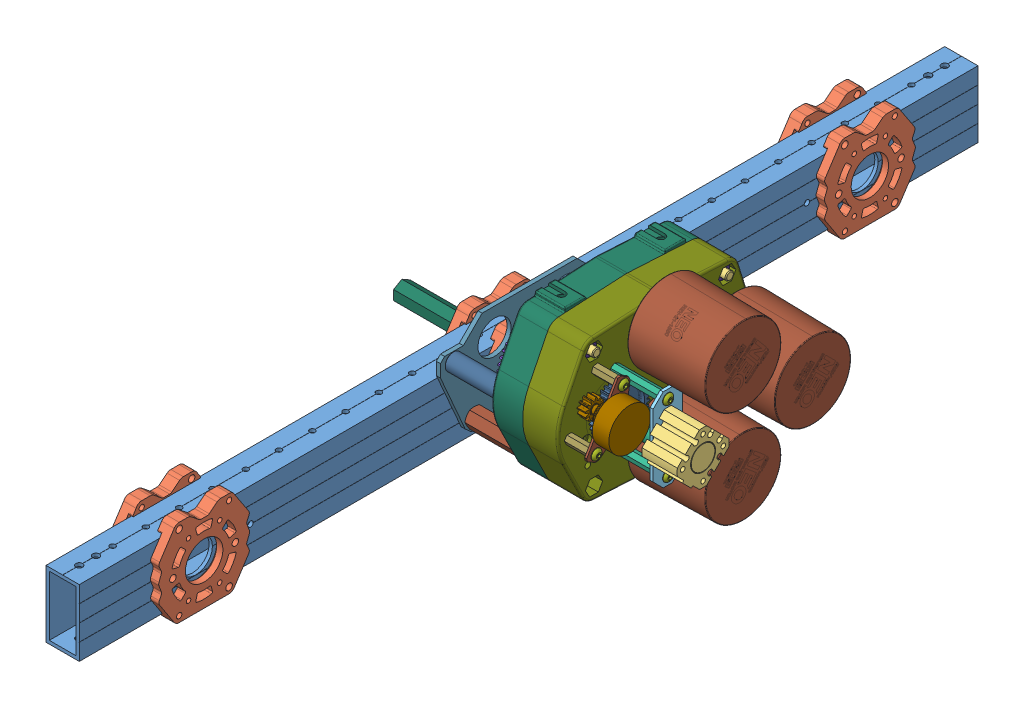
SolidWorks assembly Copy of 2020IR.subassembly_drivebase_gearbox_wheels_mounted.originaldownload.osears, configuration Default. Lengths in mm.
Overall size (265.36 166.93 685.8).
117 component instances, 65 part files, 0 mates.
Components (placement in the parent):
- 217-8000-001-002_mod_to_1_x_2_x_0_100_Pre-Drilled_VersaFrame_Aluminum_Tube_(27)_217-3453.drp-1: 217-8000-001-002_mod_to_1_x_2_x_0_100_Pre-Drilled_VersaFrame_Aluminum_Tube_(27)_217-3453.drp [Default] at (-12.7 22.86 749.3) size (25.4 50.8 685.8)
- VersaBlock_Kit_217-3432.drp-1: VersaBlock_Kit_217-3432.drp [Default] at (1.5875 24.5237 596.8746) x (0 0 -1) z (1 0 0) size (69.4 66.32 9.53)
- VersaBlock_Kit_217-3432.drp-2: VersaBlock_Kit_217-3432.drp [Default] at (1.5875 24.5237 342.8746) x (0 0 -1) z (1 0 0) size (69.4 66.32 9.53)
- VersaBlock_Kit_217-3432.drp-3: VersaBlock_Kit_217-3432.drp [Default] at (1.5875 24.5237 88.8746) x (0 0 -1) z (1 0 0) size (69.4 66.32 9.53)
- VersaBlock_Kit_217-3432.drp-4: VersaBlock_Kit_217-3432.drp [Default] at (-26.9875 24.5237 88.8746) x (0 0 1) z (-1 0 0) size (69.4 66.32 9.53)
- VersaBlock_Kit_217-3432.drp-5: VersaBlock_Kit_217-3432.drp [Default] at (-26.9875 24.5237 342.8746) x (0 0 1) z (-1 0 0) size (69.4 66.32 9.53)
- VersaBlock_Kit_217-3432.drp-6: VersaBlock_Kit_217-3432.drp [Default] at (-26.9875 24.5237 596.8746) x (0 0 1) z (-1 0 0) size (69.4 66.32 9.53)
- 3_CIM_Ball_Shifter_Base_Kit_with_WCD_3rd_Stage_217-3269_With_NEO.drp-1: 3_CIM_Ball_Shifter_Base_Kit_with_WCD_3rd_Stage_217-3269_With_NEO.drp [Default] at (101.2952 62.8142 378.4138) x (0 1 0) z (-1 0 0) size (166.93 180.09 265.36)
  - 3_CIM_Ball_Shifter_Base_Kit_with_WCD_3rd_Stage_217-3269.STEP-1: 3_CIM_Ball_Shifter_Base_Kit_with_WCD_3rd_Stage_217-3269.STEP [Default] at origin size (154.62 161.2 265.36)
    - 217-2778-001 Rev2_NCQ8A075-050M.STEP-1: 217-2778-001 Rev2_NCQ8A075-050M.STEP [Default] at (0 0 -53.848) x (-0.707107 0.707107 0) z (0 0 1) size (31.75 33.34 39.88)
      - 217-2778-NCQ8A075-050M_NCQ8 Tube_075A.STEP-1: 217-2778-NCQ8A075-050M_NCQ8 Tube_075A.STEP [Default] at origin size (31.75 33.34 26.92)
      - 217-2778-NCQ8A075-050M_NCQ8 Rod_075M.STEP-1: 217-2778-NCQ8A075-050M_NCQ8 Rod_075M.STEP [Default] at (0 0 -8.85) x (0.866025 -0.5 0) z (0 0 1) size (18.95 18.95 35.27)
      - 217-2778-NCQ8A075-050M_Snap Ring_075.STEP-1: 217-2778-NCQ8A075-050M_Snap Ring_075.STEP [Default] at (0 0 10.362) size (21 20.74 0.97)
    - 217-4098-100 Rev1.STEP-1: 217-4098-100 Rev1.STEP [Default] at (0 0 -16.927) x (-0.503316 0.864103 0) z (0 0 1) size (18.03 19.79 22.46)
      - 217-4098-006 Rev2.STEP-1: 217-4098-006 Rev2.STEP [Default] at (0 0 -4.6312) x (0 -1 0) z (0 0 -1) size (18.09 11.02 22.46)
      - 217-4098-006 Rev2.STEP-2: 217-4098-006 Rev2.STEP [Default] at (0 0 -4.6312) x (0 1 0) z (0 0 -1) size (18.09 11.02 22.46)
      - 217-3489-001 Rev1.STEP-1: 217-3489-001 Rev1.STEP [Default] at (0 0 -4.6312) x (0 0 1) z (-0.980217 -0.197926 0) size (4.77 12.7 12.7)
      - 97633A130_97633A130_grv.STEP-1: 97633A130_97633A130_grv.STEP [Default] at (0 0 -7.33) x (0 0 -1) z (0.979861 0.199683 0) size (0.64 8.74 7.34)
      - 91251A107_91251A107.STEP-1: 91251A107_91251A107.STEP [Default] at (-4.8375 -6.735 -9.4343) x (0 0.863883 -0.503692) z (-1 0 0) size (4.65 4.65 10.79)
      - 91251A107_91251A107.STEP-2: 91251A107_91251A107.STEP [Default] at (4.8375 6.735 -9.4343) x (0 0.470889 -0.882193) z (1 0 0) size (4.65 4.65 10.79)
    - 217-3288-001 Rev3.STEP-1: 217-3288-001 Rev3.STEP [Default] at (0 0 0.0889) x (0.055929 -0.998435 0) z (0 0 1) size (99.51 99.53 98.3)
      - 217-4099-000 Rev2_high gear.STEP-1: 217-4099-000 Rev2_high gear.STEP [Default] x (-1 0 0) z (0 0 1) size (22.23 22.23 98.3)
        - 217-4098-005 Rev1_91612A226.STEP-1: 217-4098-005 Rev1_91612A226.STEP [Default] at (0 0 46.2661) x (-0.144757 0 0.989467) z (0 -1 0) size (3.02 3.15 18.22)
        - 217-4098-003 Rev2.STEP-1: 217-4098-003 Rev2.STEP [Default] x (1 0 0) z (0 0 -1) size (22.23 22.23 55.94)
        - 217-4099-002 Rev3.STEP-1: 217-4099-002 Rev3.STEP [Default] at (0 0 53.467) x (0 0 1) z (-1 0 0) size (40.96 12.73 14.67)
        - 217-4098-004 Rev1.STEP-1: 217-4098-004 Rev1.STEP [Default] at (0 0 14.2494) x (0.873474 -0.48687 0) z (0 0 1) size (11.68 11.68 56)
      - 217-3212-101 Rev1.STEP-1: 217-3212-101 Rev1.STEP [Default] at (-11.5751 10.4131 45.3224) x (0.923728 0.383049 0) z (0 0 -1) size (46.46 46.56 12.7)
        - 217-2428-022 Rev1.STEP-1: 217-2428-022 Rev1.STEP [Default] at (6.7035 14.0527 24.6087) size (28.57 28.57 6.1)
        - 217-3212-001 Rev1_34t.STEP-1: 217-3212-001 Rev1_34t.STEP [Default] at (6.7035 14.0527 27.9107) size (46.46 46.56 11.11)
      - 217-3222-101 Rev1.STEP-1: 217-3222-101 Rev1.STEP [Default] at (21.0941 -5.2804 52.7371) x (-0.889163 -0.457591 0) z (0 0 -1) size (73.87 73.92 12.7)
        - 217-2428-022 Rev1.STEP-1: 217-2428-022 Rev1.STEP [Default] at (16.3398 14.3476 19.3234) size (28.57 28.57 6.1)
        - 217-3222-001 Rev1_Spur01.STEP-1: 217-3222-001 Rev1_Spur01.STEP [Default] at (16.3398 14.3476 22.6254) x (0.999377 0.0353 0) z (0 0 1) size (71.39 71.45 11.11)
      - 217-2428-008 Rev2.STEP-1: 217-2428-008 Rev2.STEP [Default] at (0 0 10.2679) size (31.75 31.75 1.59)
      - 217-2428-028 Rev1_97633A250.STEP-1: 217-2428-028 Rev1_97633A250.STEP [Default] at (0 0 37.1221) x (0 0 1) z (0.9357 -0.352797 0) size (1.07 23.39 21.18)
      - 217-2428-007 Rev1.STEP-1: 217-2428-007 Rev1.STEP [Default] at (7.809 4.5085 14.2494) x (-0.69071 0.455693 -0.561483) z (-0.67559 -0.683536 0.276329) size (6.35 6.35 6.35)
      - 217-2428-007 Rev1.STEP-2: 217-2428-007 Rev1.STEP [Default] at (5.4343 3.1375 26.9494) x (-0.162331 -0.978398 0.128005) z (0.857281 -0.204076 -0.472676) size (6.35 6.35 6.35)
      - 217-2428-007 Rev1.STEP-3: 217-2428-007 Rev1.STEP [Default] at (-5.4343 3.1375 26.9494) x (0.928483 0.348617 0.128005) z (-0.251905 0.844465 -0.472676) size (6.35 6.35 6.35)
      - 217-2428-007 Rev1.STEP-4: 217-2428-007 Rev1.STEP [Default] at (0 -6.275 26.9494) x (-0.766153 0.629782 0.128005) z (-0.605376 -0.640389 -0.472676) size (6.35 6.35 6.35)
      - 217-2428-007 Rev1.STEP-5: 217-2428-007 Rev1.STEP [Default] at (-7.809 4.5085 14.2494) x (-0.049287 -0.826019 -0.561483) z (0.929754 -0.24331 0.276329) size (6.35 6.35 6.35)
      - 217-2428-007 Rev1.STEP-6: 217-2428-007 Rev1.STEP [Default] at (0 -9.017 14.2494) x (0.739997 0.370326 -0.561483) z (-0.254164 0.926846 0.276329) size (6.35 6.35 6.35)
    - 217-2733-001 Rev2.STEP-1: 217-2733-001 Rev2.STEP [Default] at (0 53.4162 37.6682) x (0 0 1) z (-0.00054 -1 0) size (7.11 24.61 24.61)
    - 217-2733-001 Rev2.STEP-2: 217-2733-001 Rev2.STEP [Default] at (0 53.4162 7.9248) x (0 0 -1) z (-0.038475 0.99926 0) size (7.11 24.61 24.61)
    - 217-2731-001 Rev2.STEP-1: 217-2731-001 Rev2.STEP [Default] at (0 0 0.0381) x (-0.099212 0.995066 0) z (0.995066 0.099212 0) size (31.12 7.94 31.12)
    - 217-2789-001 Rev2.STEP-1: 217-2789-001 Rev2.STEP [Default] at (0 0 43.2943) x (0 0 -1) z (-0.58471 0.811243 0) size (11.1 38.4 38.4)
    - 217-2428-012 Rev2.STEP-1: 217-2428-012 Rev2.STEP [Default] at (0 0 -40.386) size (63.5 22.23 2.29)
    - 217-2428-005 Rev1.STEP-1: 217-2428-005 Rev1.STEP [Default] at (25.4 0 -19.05) x (-0.557362 -0.83027 0) z (-0.83027 0.557362 0) size (7.33 38.98 6.35)
    - 217-2428-005 Rev1.STEP-2: 217-2428-005 Rev1.STEP [Default] at (-25.4 0 -19.05) x (0.667436 0.744667 0) z (0.744667 -0.667436 0) size (7.33 38.98 6.35)
    - SCREW-832-0375.STEP-1: SCREW-832-0375.STEP [Default] at (25.4 0 -42.5958) x (0 0 1) z (-0.875404 0.483392 0) size (11.73 7.92 7.92)
    - SCREW-832-0375.STEP-2: SCREW-832-0375.STEP [Default] at (-25.4 0 -42.5958) x (0 0 1) z (-0.966319 0.257347 0) size (11.73 7.92 7.92)
    - SCREW-832-0375.STEP-3: SCREW-832-0375.STEP [Default] at (25.4 0 5.3848) x (0 0 -1) z (1 0 0) size (11.73 7.92 7.92)
    - SCREW-832-0375.STEP-4: SCREW-832-0375.STEP [Default] at (-25.4 0 5.3848) x (0 0 -1) z (0.941463 -0.337115 0) size (11.73 7.92 7.92)
    - SBS1_SBS-0632-0250.STEP-1: SBS1_SBS-0632-0250.STEP [Default] at (15.494 0 -36.2458) x (0 0 -1) z (0.854303 -0.519775 0) size (8.57 6.68 6.65)
    - SBS1_SBS-0632-0250.STEP-2: SBS1_SBS-0632-0250.STEP [Default] at (-15.494 0 -36.2458) x (0 0 -1) z (0.854303 -0.519775 0) size (8.57 6.68 6.65)
    - 217-2428-017 Rev2.STEP-1: 217-2428-017 Rev2.STEP [Default] at (12.7 -21.997 -3.614) x (-0.578458 -0.815712 0) z (0 0 -1) size (14.73 14.73 7.37)
    - 217-2428-016 Rev3_Spur01.STEP-1: 217-2428-016 Rev3_Spur01.STEP [Default] at (0 0 -3.614) x (0.873157 -0.48744 0) z (0 0 1) size (40.67 40.74 13.32)
    - 217-2428-019 Rev1.STEP-1: 217-2428-019 Rev1.STEP [Default] at (12.7 -21.997 -20.6248) x (0.866025 0.5 0) z (0 0 1) size (50.8 19.05 1.57)
    - 217-2428-006 Rev1.STEP-1: 217-2428-006 Rev1.STEP [Default] at (32.079 -14.2875 -9.525) x (-0.752416 0.658689 0) z (0.658689 0.752416 0) size (7.33 19.93 6.35)
    - 217-2428-006 Rev1.STEP-2: 217-2428-006 Rev1.STEP [Default] at (-3.6662 -34.925 -9.525) x (0.84498 0.534798 0) z (0.534798 -0.84498 0) size (7.33 19.93 6.35)
    - SCREW-832-0375.STEP-5: SCREW-832-0375.STEP [Default] at (32.079 -14.2875 4.7498) x (0 0 -1) z (0.980613 0.195955 0) size (11.73 7.92 7.92)
    - SCREW-832-0375.STEP-6: SCREW-832-0375.STEP [Default] at (-3.6662 -34.925 5.3848) x (0 0 -1) z (-0.672515 -0.740083 0) size (11.73 7.92 7.92)
    - SCREW-832-0375.STEP-7: SCREW-832-0375.STEP [Default] at (-3.6662 -34.925 -22.8346) x (0 0 1) z (0.948865 0.315681 0) size (11.73 7.92 7.92)
    - SCREW-832-0375.STEP-8: SCREW-832-0375.STEP [Default] at (32.079 -14.2875 -22.8346) x (0 0 1) z (-0.875404 0.483392 0) size (11.73 7.92 7.92)
    - 217-2614-001_12t.STEP-1: 217-2614-001_12t.STEP [Default] at (36.9798 39.6868 15.8623) x (-0.087156 0.996195 0) z (0 0 1) size (18.29 18.29 19)
    - 217-2761-001 rev1.STEP-1: 217-2761-001 rev1.STEP [Default] at (33.1943 39.3556 16.1) x (0.087156 -0.996195 0) z (0 0 1) size (2 2 20)
    - 217-2761-001 rev1.STEP-2: 217-2761-001 rev1.STEP [Default] at (-40.7653 40.018 16.1) x (0.087156 0.996195 0) z (0 0 1) size (2 2 20)
    - 217-2614-001_12t.STEP-2: 217-2614-001_12t.STEP [Default] at (-36.9798 39.6868 15.8623) x (0.087156 0.996195 0) z (0 0 1) size (18.29 18.29 19)
    - 217-2614-001_12t.STEP-3: 217-2614-001_12t.STEP [Default] at (0 92.8624 15.8623) x (0.97459 0.223996 0) z (0 0 1) size (18.29 18.29 19)
    - 217-2761-001 rev1.STEP-3: 217-2761-001 rev1.STEP [Default] at (-0.8512 96.5658 16.1) x (0.97459 0.223996 0) z (0 0 1) size (2 2 20)
    - 217-3195-002 rev2.STEP-1: 217-3195-002 rev2.STEP [Default] at (0 0 50.546) x (-1 0 0) z (0 0 -1) size (114.31 152.24 24.96)
    - 217-3195-001 Rev1.STEP-1: 217-3195-001 Rev1.STEP [Default] at origin size (113.41 152.24 26.86)
    - Nylock Nut_NNY2520-ZC.STEP-1: Nylock Nut_NNY2520-ZC.STEP [Default] at (48.8823 73.025 37.846) x (0 0.866025 -0.5) z (-1 0 0) size (12.85 11.89 7.62)
    - Nylock Nut_NNY2520-ZC.STEP-2: Nylock Nut_NNY2520-ZC.STEP [Default] at (48.8823 -3.175 37.846) x (0 0 -1) z (-1 0 0) size (12.85 11.89 7.62)
    - Nylock Nut_NNY2520-ZC.STEP-3: Nylock Nut_NNY2520-ZC.STEP [Default] at (44.45 85.725 7.8613) x (0 1 0) z (0 0 -1) size (12.85 11.89 7.62)
    - 276-1027-001.STEP-1: 276-1027-001.STEP [Default] at (47.625 58.1787 6.35) x (0 1 0) z (-1 0 0) size (8.61 5.64 9.94)
    - 276-1027-001.STEP-2: 276-1027-001.STEP [Default] at (-47.625 58.1787 6.35) x (0 -1 0) z (1 0 0) size (8.61 5.64 9.94)
    - SCREW-832-1750.STEP-1: SCREW-832-1750.STEP [Default] at (-47.625 58.1787 47.0408) x (0 0 -1) z (-0.960822 -0.277167 0) size (46.66 7.92 7.92)
    - SCREW-832-1750.STEP-2: SCREW-832-1750.STEP [Default] at (47.625 58.1787 47.0408) x (0 0 -1) z (-0.960822 -0.277167 0) size (46.66 7.92 7.92)
    - Nylock Nut_NNY2520-ZC.STEP-4: Nylock Nut_NNY2520-ZC.STEP [Default] at (44.45 -15.875 7.8613) x (0 1 0) z (0 0 -1) size (12.85 11.89 7.62)
    - 217-2428-004 Rev3.STEP-1: 217-2428-004 Rev3.STEP [Default] at (0 53.4162 22.7711) x (-0.709585 0.70462 0) z (0 0 1) size (11 9.53 43.92)
    - SBS1_SBS-2520-1625SS.STEP-1: SBS1_SBS-2520-1625SS.STEP [Default] at (44.45 85.725 42.4688) x (0 0 -1) z (-0.251219 0.96793 0) size (45.3 11.2 11.18)
    - SBS1_SBS-2520-1625SS.STEP-2: SBS1_SBS-2520-1625SS.STEP [Default] at (44.45 -15.875 42.4688) x (0 0 -1) z (-0.251219 0.96793 0) size (45.3 11.2 11.18)
    - SBS1_SBS2520-1750.STEP-1: SBS1_SBS2520-1750.STEP [Default] at (-44.45 85.725 7.4422) x (0 0 1) z (-0.031478 0.999504 0) size (48.48 11.2 11.18)
    - SBS1_SBS2520-1750.STEP-2: SBS1_SBS2520-1750.STEP [Default] at (-44.45 -15.875 7.4422) x (0 0 1) z (-0.937114 -0.349025 0) size (48.48 11.2 11.18)
    - 217-2428-021 Rev1.STEP-1: 217-2428-021 Rev1.STEP [Default] at (0 53.4162 9.5123) x (0.451333 -0.892356 0) z (0 0 1) size (15.88 15.88 3.17)
    - 217-2428-029 Rev1.STEP-1: 217-2428-029 Rev1.STEP [Default] at (0 53.4162 36.957) x (0.999846 0.017557 0) z (0 0 1) size (15.88 15.88 1.12)
    - Grayhill Lock Washer.STEP-1: Grayhill Lock Washer.STEP [Default] at (12.7 -21.997 -18.6817) x (0.467173 -0.884166 0) z (0 0 1) size (19.69 19.69 0.74)
    - Grayhill Nut.STEP-1: Grayhill Nut.STEP [Default] at (12.7 -21.997 -17.0434) x (0.984088 0.177684 0) z (0 0 1) size (18.33 15.88 2.54)
    - Grahill Encoder.STEP-1: Grahill Encoder.STEP [Default] at (12.7 -21.997 -16.1798) x (-0.580071 0.814566 0) z (-0.814566 -0.580071 0) size (31.75 31.12 31.75)
    - 217-3195-009 Rev1_wcd 2.STEP-1: 217-3195-009 Rev1_wcd 2.STEP [Default] at (0 85.725 50.546) x (-0.998427 -0.056065 0) z (0 0 1) size (12.7 12.7 41.27)
    - 217-3195-006 Rev1_WCD.STEP-1: 217-3195-006 Rev1_WCD.STEP [Default] at (-44.45 85.725 44.1452) x (0.5 0.866025 0) z (0 0 1) size (12.7 14.66 47.62)
    - 217-3195-009 Rev1_wcd 2.STEP-2: 217-3195-009 Rev1_wcd 2.STEP [Default] at (0 -31.75 50.546) x (0.947633 0.319361 0) z (0 0 1) size (12.7 12.7 41.27)
    - 217-3195-006 Rev1_WCD.STEP-2: 217-3195-006 Rev1_WCD.STEP [Default] at (-44.45 -15.875 44.1452) x (0.5 -0.866025 0) z (0 0 1) size (12.7 14.66 47.62)
    - Nylock Nut_NNY2520-ZC.STEP-5: Nylock Nut_NNY2520-ZC.STEP [Default] at (0 -31.75 45.0723) x (-0.5 0.866025 0) z (0 0 -1) size (12.85 11.89 7.62)
    - Nylock Nut_NNY2520-ZC.STEP-6: Nylock Nut_NNY2520-ZC.STEP [Default] at (0 85.725 45.0723) x (-0.5 0.866025 0) z (0 0 -1) size (12.85 11.89 7.62)
    - SBS1_SBS-2520-2250.STEP-1: SBS1_SBS-2520-2250.STEP [Default] at (0 -31.75 98.298) x (0 0 -1) z (-0.933488 -0.358607 0) size (61.18 11.22 11.17)
    - SBS1_SBS2520-0625ZC.STEP-1: SBS1_SBS2520-0625ZC.STEP [Default] at (-44.45 85.725 98.298) x (0 0 -1) z (0.400817 0.916158 0) size (19.57 11.22 11.17)
    - SBS1_SBS2520-0625ZC.STEP-2: SBS1_SBS2520-0625ZC.STEP [Default] at (-44.45 -15.875 98.298) x (0 0 -1) z (-0.75178 -0.659414 0) size (19.57 11.22 11.17)
    - SBS1_SBS-2520-2250.STEP-2: SBS1_SBS-2520-2250.STEP [Default] at (0 85.725 98.298) x (0 0 -1) z (0.056677 -0.998393 0) size (61.18 11.22 11.17)
    - 217-3195-003 rev2.STEP-1: 217-3195-003 rev2.STEP [Default] at (0 0 94.9452) size (88.62 139.7 3.17)
    - 217-2617-003 Rev1.STEP-1: 217-2617-003 Rev1.STEP [Default] at (-39.878 35.5392 121.8535) x (-0.5 -0.866025 0) z (0 0 1) size (14.66 12.7 152.4)
    - 217-3109-001 Rev1.STEP-1: 217-3109-001 Rev1.STEP [Default] at (-39.878 35.5392 49.1808) x (0 0 1) z (0.312889 -0.94979 0) size (7.94 28.57 28.57)
    - 217-2734-001 Rev3.STEP-1: 217-2734-001 Rev3.STEP [Default] at (-39.878 35.5392 98.1202) x (1 0 0) z (0 1 0) size (31.12 7.94 31.12)
    - 217-2617-004 Rev1_97431A340_grv.STEP-1: 217-2617-004 Rev1_97431A340_grv.STEP [Default] at (-39.878 35.5392 54.8961) x (0 0 1) z (-0.124043 -0.992277 0) size (1.07 20.42 18.58)
    - 217-2617-004 Rev1_97431A340_grv.STEP-2: 217-2617-004 Rev1_97431A340_grv.STEP [Default] at (0 0 69.215) x (0 0 1) z (-0.124043 -0.992277 0) size (1.07 20.42 18.58)
    - 217-2702-001_20t.STEP-1: 217-2702-001_20t.STEP [Default] at (0 0 62.357) x (0.998435 0.055929 0) z (0 0 1) size (28.2 28.2 12.65)
    - 217-2715-002 Rev1_64t.STEP-1: 217-2715-002 Rev1_64t.STEP [Default] at (-39.878 35.5392 61.7541) x (0.866025 -0.5 0) z (0 0 1) size (84.3 84.3 12.65)
    - 217-2704-001_24.STEP-1: 217-2704-001_24.STEP [Default] at (0 0 62.357) x (0.450781 0.892635 0) z (0 0 -1) size (33.29 33.29 12.65)
    - 217-2714-002 Rev1_60t.STEP-1: 217-2714-002 Rev1_60t.STEP [Default] at (-39.878 35.5392 61.7541) x (0.866025 -0.5 0) z (0 0 1) size (78.95 78.95 12.65)
    - 217-3221-002 Rev1.STEP-1: 217-3221-002 Rev1.STEP [Default] at (-39.878 35.5392 61.7414) x (0 -1 0) z (0 0 1) size (71.39 71.45 12.62)
    - 217-2705-001_30t.STEP-1: 217-2705-001_30t.STEP [Default] at (0 0 62.357) x (0.547654 -0.836705 0) z (0 0 1) size (41.01 41.12 12.65)
    - 217-2712-002 Rev1_50t.STEP-1: 217-2712-002 Rev1_50t.STEP [Default] at (-39.878 35.5392 61.7541) x (0.866025 -0.5 0) z (0 0 1) size (66.7 66.76 12.65)
    - 217-2706-001_34t.STEP-1: 217-2706-001_34t.STEP [Default] at (0 0 62.357) x (0.998435 0.055929 0) z (0 0 1) size (46.46 46.56 12.65)
    - 217-3210-001 Rev1_30t.STEP-1: 217-3210-001 Rev1_30t.STEP [Default] at (0 53.4162 30.0736) x (-0.966828 0.255427 0) z (0 0 1) size (41.01 41.12 12.65)
    - 217-2711-002 Rev1_50t.STEP-1: 217-2711-002 Rev1_50t.STEP [Default] at (0 53.4162 17.4244) x (0.262208 -0.965011 0) z (0 0 1) size (66.7 66.76 12.65)
  - REV-21-1650 (1).step-1: REV-21-1650 (1).step [Default] at (0 92.8624 0) size (64.41 64.76 93.26)
  - REV-21-1650 (1).step-2: REV-21-1650 (1).step [Default] at (36.9798 39.6868 0) x (0.996195 0.087156 0) z (0 0 1) size (64.41 64.76 93.26)
  - REV-21-1650 (1).step-3: REV-21-1650 (1).step [Default] at (-36.9798 39.6868 0) x (0.996195 -0.087156 0) z (0 0 1) size (64.41 64.76 93.26)
